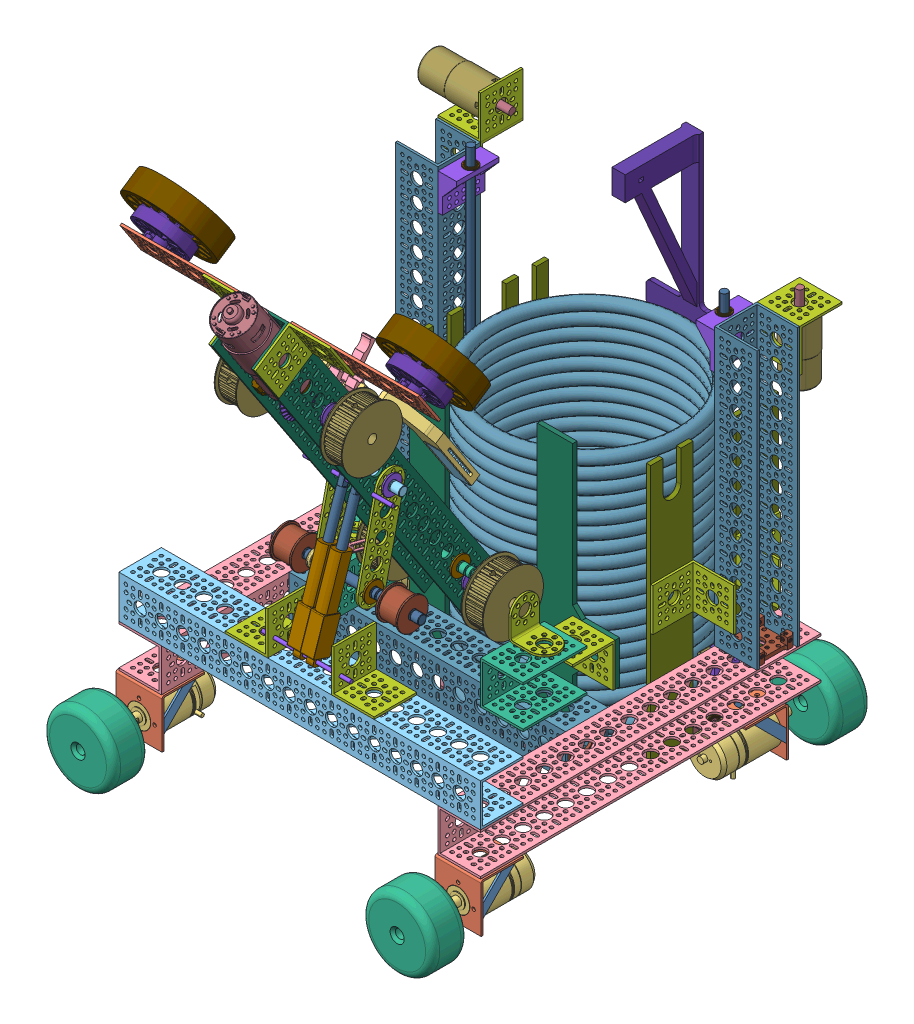
SolidWorks assembly 底座3.5, configuration 默认. Lengths in mm. (continued)
Mates (geometry in assembly coordinates): (continued)
- Concentric323: concentric aligned: cylinder of 升降轴-1 through (7.3414 252.9349 701.0171) axis (-1 0 0) radius 2; cylinder of 电动推杆01-1 through (-46.1586 252.9349 701.0171) axis (-1 0 0) radius 2
- Concentric324: concentric aligned: cylinder of 升降轴-1 through (7.3414 252.9349 701.0171) axis (-1 0 0) radius 2; cylinder of 电动推杆01-2 through (-31.1586 252.9349 701.0171) axis (-1 0 0) radius 2
- Concentric325: concentric anti-aligned: cylinder of 电动推杆01-2 through (-35.1586 294.1889 687.2204) axis (0 0.94837 -0.317167) radius 4.5; cylinder of 电动推杆2-1 through (-35.1586 393.1181 654.1351) axis (0 -0.94837 0.317167) radius 4.5
- LimitDistance1: limit distance = 5.6851 mm anti-aligned: plane of 电动推杆2-1 through (-35.1586 340.9577 671.5793) normal (0 -0.94837 0.317167); plane of 电动推杆01-2 through (-35.1586 346.3493 669.7762) normal (0 0.94837 -0.317167)
- LimitDistance2: limit distance = 49.3149 mm aligned: plane of 电动推杆2-1 through (-35.1586 393.1181 654.1351) normal (0 0.94837 -0.317167); plane of 电动推杆01-2 through (-35.1586 346.3493 669.7762) normal (0 0.94837 -0.317167)
- Concentric328: concentric anti-aligned: cylinder of 电动推杆01-1 through (-50.1586 294.1889 687.2204) axis (0 0.94837 -0.317167) radius 4.5; cylinder of 电动推杆2-2 through (-50.1586 393.1181 654.1351) axis (0 -0.94837 0.317167) radius 4.5
- LimitDistance6: limit distance = 5.6851 mm anti-aligned: plane of 电动推杆01-1 through (-50.1586 346.3493 669.7762) normal (0 0.94837 -0.317167); plane of 电动推杆2-2 through (-50.1586 340.9577 671.5793) normal (0 -0.94837 0.317167)
- LimitDistance7: limit distance = 49.3149 mm aligned: plane of 电动推杆2-2 through (-50.1586 393.1181 654.1351) normal (0 0.94837 -0.317167); plane of 电动推杆01-1 through (-50.1586 346.3493 669.7762) normal (0 0.94837 -0.317167)
- Coincident131: coincident anti-aligned: plane of 电动推杆01-1 through (-42.6586 291.0173 677.7367) normal (1 0 0); plane of 电动推杆01-2 through (-42.6586 297.3606 696.7041) normal (-1 0 0)
- Distance12: distance = 21 mm anti-aligned: plane of 电动推杆01-1 through (-57.6586 297.3606 696.7041) normal (-1 0 0); plane of 48x48-L形支架-3 through (-78.6586 237.4201 661.5024) normal (1 0 0)
- Coincident286: coincident anti-aligned: plane of 384mm-U型梁-2 through (161.3414 189.4201 325.5024) normal (0 1 0); plane of 电机转向座-9 through (137.3414 189.4201 373.5024) normal (0 -1 0)
- Concentric623: concentric anti-aligned: cylinder of 48x48-L形支架-17 through (137.3414 491.4201 325.5024) axis (0 1 0) radius 7; cylinder of 一级摩擦轮电机01-2 through (137.3414 498.9201 325.5024) axis (0 -1 0) radius 11
- Coincident301: coincident anti-aligned: plane of 48x48-L形支架-17 through (113.3414 498.9201 347.0024) normal (0 -1 0); plane of 一级摩擦轮电机01-2 through (137.3414 498.9201 325.5024) normal (0 1 0)
- Tangent10: tangent anti-aligned: plane of 48x48-L形支架-17 through (135.3414 491.4201 347.0024) normal (1 0 0); cylinder of 一级摩擦轮电机01-2 through (136.8414 491.6201 311.5113) axis (0 1 0) radius 1.5
- Concentric624: concentric anti-aligned: cylinder of 一级摩擦轮电机01-2 through (137.3414 495.9201 325.5024) axis (0 1 0) radius 4; cylinder of 一级摩擦轮电机02-2 through (137.3414 515.9201 325.5024) axis (0 -1 0) radius 4
- Coincident302: coincident anti-aligned: plane of 一级摩擦轮电机01-2 through (137.3414 495.9201 325.5024) normal (0 1 0); plane of 一级摩擦轮电机02-2 through (137.3414 495.9201 325.5024) normal (0 -1 0)
- Concentric637: concentric aligned: cylinder of 384mm-U型梁-1 through (-222.6586 179.4201 373.5024) axis (0 1 0) radius 7; cylinder of 电机转向座-12 through (-222.6586 189.4201 373.5024) axis (0 1 0) radius 7
- Concentric638: concentric aligned: cylinder of 384mm-U型梁-2 through (137.3414 179.4201 373.5024) axis (0 1 0) radius 7; cylinder of 电机转向座-9 through (137.3414 189.4201 373.5024) axis (0 1 0) radius 7
- Coincident316: coincident aligned: plane of 384mm-U型梁-2 through (161.3414 189.4201 325.5024) normal (0 1 0); plane of 312mm-U型梁-7 through (113.3414 189.4201 565.5024) normal (0 1 0)
- Coincident317: coincident anti-aligned: plane of 384mm-U型梁-2 through (113.3414 189.4201 325.5024) normal (-1 0 0); plane of 312mm-U型梁-7 through (113.3414 186.9201 541.5024) normal (1 0 0)
- Concentric650: concentric anti-aligned: cylinder of 312mm-U型梁-7 through (105.3414 179.4201 557.5024) axis (0 1 0) radius 2; cone of 电机转向座-13 through (105.3414 186.9201 557.5024) axis (0 -1 0)
- Concentric651: concentric anti-aligned: cylinder of 312mm-U型梁-7 through (105.3414 179.4201 525.5024) axis (0 1 0) radius 2; cone of 电机转向座-13 through (105.3414 186.9201 525.5024) axis (0 -1 0)
- Concentric652: concentric anti-aligned: cylinder of 312mm-U型梁-7 through (105.3414 181.4201 527.5024) axis (0 0 -1) radius 2; cone of 电机转向座-13 through (105.3414 181.4201 520.0024) axis (0 0 1)
- Concentric653: concentric anti-aligned: cylinder of 312mm-U型梁-7 through (105.3414 149.4201 527.5024) axis (0 0 -1) radius 2; cone of 电机转向座-13 through (105.3414 149.4201 520.0024) axis (0 0 1)
- Coincident318: coincident anti-aligned: plane of 384mm-U型梁-2 through (113.3414 189.4201 325.5024) normal (-1 0 0); plane of 电机转向座-13 through (113.3414 165.4201 541.5024) normal (1 0 0)
- Concentric654: concentric aligned: cylinder of 384mm-U型梁-2 through (123.3414 165.4201 541.5024) axis (-1 0 0) radius 7; cylinder of 电机转向座-13 through (113.3414 165.4201 541.5024) axis (-1 0 0) radius 7
- Concentric655: concentric aligned: cylinder of 384mm-U型梁-2 through (123.3414 156.9349 533.0171) axis (-1 0 0) radius 2; cylinder of 电机转向座-13 through (109.3414 156.9349 533.0171) axis (-1 0 0) radius 2
- Concentric661: concentric anti-aligned: cylinder of 312mm-U型梁-7 through (65.3414 179.4201 541.5024) axis (0 1 0) radius 7; cylinder of 72mm-U型梁-5 through (65.3414 199.4201 541.5024) axis (0 -1 0) radius 7
- Coincident323: coincident anti-aligned: plane of 312mm-U型梁-7 through (113.3414 189.4201 565.5024) normal (0 1 0); plane of 72mm-U型梁-5 through (89.3414 189.4201 589.5024) normal (0 -1 0)
- Concentric662: concentric anti-aligned: cylinder of 312mm-U型梁-7 through (81.3414 179.4201 557.5024) axis (0 1 0) radius 2; cylinder of 72mm-U型梁-5 through (81.3414 199.4201 557.5024) axis (0 -1 0) radius 2
- Coincident324: coincident anti-aligned: plane of 312mm-U型梁-7 through (113.3414 189.4201 565.5024) normal (0 1 0); plane of 72mm-U型梁-6 through (-174.6586 189.4201 589.5024) normal (0 -1 0)
- Concentric666: concentric aligned: cylinder of 72mm-U型梁-5 through (65.3414 227.4201 541.5024) axis (0 1 0) radius 7; cylinder of 圆角90°法兰-7 through (65.3414 237.4201 541.5024) axis (0 1 0) radius 7
- Coincident325: coincident anti-aligned: plane of 72mm-U型梁-5 through (89.3414 237.4201 589.5024) normal (0 1 0); plane of 圆角90°法兰-7 through (41.3414 237.4201 557.5024) normal (0 -1 0)
- Concentric667: concentric aligned: cylinder of 72mm-U型梁-5 through (54.0277 234.4201 541.5024) axis (0 1 0) radius 2; cylinder of 圆角90°法兰-7 through (54.0277 237.4201 541.5024) axis (0 1 0) radius 2.025
- Coincident326: coincident anti-aligned: plane of 72mm-U型梁-6 through (-174.6586 237.4201 589.5024) normal (0 1 0); plane of 圆角90°法兰-8 through (-126.6586 237.4201 525.5024) normal (0 -1 0)
- Concentric670: concentric anti-aligned: cylinder of 总装-2/同步轮四十齿(1)-3 through (30.3158 261.4201 541.5024) axis (-1 0 0) radius 5; cylinder of 圆角90°法兰-7 through (41.3414 261.4201 541.5024) axis (1 0 0) radius 7
- Distance14: distance = 12.71 mm anti-aligned: plane of 总装-2/同步轮四十齿(1)-1 through (-113.9486 261.4201 541.5024) normal (-1 0 0); plane of 圆角90°法兰-8 through (-126.6586 237.4201 525.5024) normal (1 0 0)
- Concentric673: concentric anti-aligned: circle of 电动推杆2-1; cylinder of 升降轴-2 through (5.3414 399.2825 652.0735) axis (-1 0 0) radius 2
- Concentric674: concentric anti-aligned: circle of 电动推杆2-2; cylinder of 升降轴-2 through (5.3414 399.2825 652.0735) axis (-1 0 0) radius 2
- Concentric675: concentric aligned: cylinder of 升降轴-2 through (5.3414 399.2825 652.0735) axis (-1 0 0) radius 2; cylinder of 总装-2/432mm-U型梁-1 through (-55.4486 399.2825 652.0735) axis (-1 0 0) radius 2
- Coincident329: coincident anti-aligned: plane of 384mm-U型梁-1 through (-246.6586 189.4201 325.5024) normal (0 1 0); plane of 电机转向座-12 through (-222.6586 189.4201 373.5024) normal (0 -1 0)
- Concentric678: concentric aligned: cylinder of 轴承座-1 through (100.3414 497.4201 373.5024) axis (0 -1 0) radius 7; cylinder of 8-14轴承-7 through (100.3414 497.4201 373.5024) axis (0 -1 0) radius 7
- Coincident330: coincident anti-aligned: plane of 轴承座-1 through (113.3414 497.4201 397.5024) normal (0 1 0); plane of 8-14轴承-7 through (100.3414 497.4201 373.5024) normal (0 -1 0)
- Coincident331: coincident anti-aligned: plane of 384mm-U型梁-2 through (113.3414 189.4201 325.5024) normal (-1 0 0); plane of 轴承座-2 through (113.3414 145.4201 397.5024) normal (1 0 0)
- Concentric679: concentric anti-aligned: cylinder of 384mm-U型梁-2 through (123.3414 181.4201 389.5024) axis (-1 0 0) radius 2; cylinder of 轴承座-2 through (95.3414 181.4201 389.5024) axis (1 0 0) radius 2.05
- Concentric680: concentric anti-aligned: cylinder of 384mm-U型梁-2 through (123.3414 181.4201 357.5024) axis (-1 0 0) radius 2; cylinder of 轴承座-2 through (95.3414 181.4201 357.5024) axis (1 0 0) radius 2.05
- Concentric681: concentric anti-aligned: cylinder of 轴承座-2 through (100.3414 145.4201 373.5024) axis (0 1 0) radius 7; cylinder of 8-14轴承-8 through (100.3414 150.4201 373.5024) axis (0 -1 0) radius 7
- Coincident332: coincident anti-aligned: plane of 轴承座-2 through (113.3414 150.4201 349.5024) normal (0 1 0); plane of 8-14轴承-8 through (100.3414 150.4201 373.5024) normal (0 -1 0)
- Concentric682: concentric anti-aligned: cylinder of 8-14轴承-8 through (100.3414 146.4201 373.5024) axis (0 1 0) radius 4; cylinder of 螺纹杆-3 through (100.3414 517.4201 373.5024) axis (0 -1 0) radius 4
- Distance15: distance = 20 mm aligned: plane of 螺纹杆-3 through (100.3414 517.4201 373.5024) normal (0 1 0); plane of 轴承座-1 through (113.3414 497.4201 397.5024) normal (0 1 0)
- Concentric684: concentric aligned: cylinder of 螺纹杆-3 through (100.3414 517.4201 373.5024) axis (0 -1 0) radius 4; cylinder of 切边螺纹滑块-1 through (100.3414 168.0411 373.5024) axis (0 -1 0) radius 3.35
- Concentric687: concentric anti-aligned: cylinder of 384mm-U型梁-1 through (-208.6586 181.4201 389.5024) axis (1 0 0) radius 2; cylinder of 轴承座-4 through (-180.6586 181.4201 389.5024) axis (-1 0 0) radius 2.05
- Concentric688: concentric anti-aligned: cylinder of 384mm-U型梁-1 through (-208.6586 181.4201 357.5024) axis (1 0 0) radius 2; cylinder of 轴承座-4 through (-180.6586 181.4201 357.5024) axis (-1 0 0) radius 2.05
- Coincident334: coincident anti-aligned: plane of 384mm-U型梁-1 through (-198.6586 141.4201 325.5024) normal (1 0 0); plane of 轴承座-4 through (-198.6586 145.4201 349.5024) normal (-1 0 0)
- Concentric689: concentric aligned: cylinder of 轴承座-3 through (-185.6586 497.4201 373.5024) axis (0 -1 0) radius 7; cylinder of 8-14轴承-9 through (-185.6586 497.4201 373.5024) axis (0 -1 0) radius 7
- Coincident335: coincident anti-aligned: plane of 轴承座-3 through (-198.6586 497.4201 349.5024) normal (0 1 0); plane of 8-14轴承-9 through (-185.6586 497.4201 373.5024) normal (0 -1 0)
- Concentric690: concentric anti-aligned: cylinder of 轴承座-4 through (-185.6586 145.4201 373.5024) axis (0 1 0) radius 7; cylinder of 8-14轴承-10 through (-185.6586 150.4201 373.5024) axis (0 -1 0) radius 7
- Coincident336: coincident anti-aligned: plane of 轴承座-4 through (-198.6586 150.4201 397.5024) normal (0 1 0); plane of 8-14轴承-10 through (-185.6586 150.4201 373.5024) normal (0 -1 0)
- Concentric691: concentric anti-aligned: cylinder of 8-14轴承-9 through (-185.6586 493.4201 373.5024) axis (0 1 0) radius 4; cylinder of 螺纹杆-4 through (-185.6586 517.4201 373.5024) axis (0 -1 0) radius 4
- Coincident337: coincident aligned: plane of 螺纹杆-3 through (100.3414 517.4201 373.5024) normal (0 1 0); plane of 螺纹杆-4 through (-185.6586 517.4201 373.5024) normal (0 1 0)
- Concentric692: concentric aligned: cylinder of 螺纹杆-4 through (-185.6586 517.4201 373.5024) axis (0 -1 0) radius 4; cylinder of 切边螺纹滑块-2 through (-185.6586 168.0411 373.5024) axis (0 -1 0) radius 3.35
- Coincident338: coincident aligned: plane of 切边螺纹滑块-1 through (100.3414 158.0411 373.5024) normal (0 1 0); plane of 切边螺纹滑块-2 through (-185.6586 158.0411 373.5024) normal (0 1 0)
- Concentric693: concentric anti-aligned: cylinder of 切边螺纹滑块-1 through (100.3414 153.0411 373.5024) axis (0 1 0) radius 5.1; cylinder of 转换块-1 through (100.3414 163.0411 373.5024) axis (0 -1 0) radius 5.5
- Concentric694: concentric aligned: cylinder of 切边螺纹滑块-1 through (100.3414 158.0411 365.5024) axis (0 -1 0) radius 1.75; cylinder of 转换块-1 through (100.3414 163.0411 365.5024) axis (0 -1 0) radius 1.75
- Coincident339: coincident anti-aligned: plane of 切边螺纹滑块-1 through (100.3414 158.0411 373.5024) normal (0 1 0); plane of 转换块-1 through (100.3414 158.0411 373.5024) normal (0 -1 0)
- Concentric695: concentric anti-aligned: cylinder of 切边螺纹滑块-2 through (-185.6586 153.0411 373.5024) axis (0 1 0) radius 5.1; cylinder of 转换块-2 through (-185.6586 163.0411 373.5024) axis (0 -1 0) radius 5.5
- Concentric696: concentric aligned: cylinder of 切边螺纹滑块-2 through (-185.6586 158.0411 365.5024) axis (0 -1 0) radius 1.75; cylinder of 转换块-2 through (-185.6586 163.0411 365.5024) axis (0 -1 0) radius 1.75
- Coincident340: coincident anti-aligned: plane of 切边螺纹滑块-2 through (-185.6586 158.0411 373.5024) normal (0 1 0); plane of 转换块-2 through (-185.6586 158.0411 373.5024) normal (0 -1 0)
- Concentric697: concentric aligned: cylinder of 384mm-U型梁-2 through (121.3414 179.4201 365.5024) axis (0 1 0) radius 2; cylinder of 电机转向座-9 through (121.3414 193.4201 365.5024) axis (0 1 0) radius 2
- Concentric698: concentric anti-aligned: cone of 电机转向座-9 through (121.3414 197.4201 352.0024) axis (0 0 1); cylinder of 312mm-U型梁-8 through (121.3414 197.4201 359.5024) axis (0 0 -1) radius 2
- Concentric699: concentric anti-aligned: cone of 电机转向座-9 through (153.3414 197.4201 352.0024) axis (0 0 1); cylinder of 312mm-U型梁-8 through (153.3414 197.4201 359.5024) axis (0 0 -1) radius 2
- Concentric700: concentric anti-aligned: cone of 电机转向座-9 through (116.1914 197.4201 357.5024) axis (1 0 0); cylinder of 312mm-U型梁-8 through (123.3414 197.4201 357.5024) axis (-1 0 0) radius 2
- Concentric701: concentric anti-aligned: cone of 电机转向座-9 through (116.1914 197.4201 389.5024) axis (1 0 0); cylinder of 312mm-U型梁-8 through (123.3414 197.4201 389.5024) axis (-1 0 0) radius 2
- Coincident341: coincident anti-aligned: plane of 轴承座-1 through (113.3414 497.4201 349.5024) normal (1 0 0); plane of 312mm-U型梁-8 through (113.3414 189.4201 349.5024) normal (-1 0 0)
- Concentric704: concentric anti-aligned: cylinder of 48x48-L形支架-17 through (153.3414 493.4201 339.5024) axis (0 0 1) radius 2; cylinder of 312mm-U型梁-8 through (153.3414 493.4201 359.5024) axis (0 0 -1) radius 2
- Concentric705: concentric anti-aligned: cylinder of 48x48-L形支架-17 through (121.3414 493.4201 339.5024) axis (0 0 1) radius 2; cylinder of 312mm-U型梁-8 through (121.3414 493.4201 359.5024) axis (0 0 -1) radius 2
- Coincident342: coincident anti-aligned: plane of 48x48-L形支架-17 through (113.3414 501.4201 349.5024) normal (0 0 1); plane of 312mm-U型梁-8 through (161.3414 189.4201 349.5024) normal (0 0 -1)
- Concentric706: concentric anti-aligned: cylinder of 轴承座-1 through (95.3414 477.4201 357.5024) axis (1 0 0) radius 2.05; cylinder of 312mm-U型梁-8 through (123.3414 477.4201 357.5024) axis (-1 0 0) radius 2
- Concentric707: concentric anti-aligned: cylinder of 轴承座-1 through (95.3414 477.4201 389.5024) axis (1 0 0) radius 2.05; cylinder of 312mm-U型梁-8 through (123.3414 477.4201 389.5024) axis (-1 0 0) radius 2
- Concentric708: concentric aligned: cylinder of 384mm-U型梁-1 through (-206.6586 179.4201 365.5024) axis (0 1 0) radius 2; cylinder of 电机转向座-12 through (-206.6586 193.4201 365.5024) axis (0 1 0) radius 2
- Concentric709: concentric anti-aligned: cone of 电机转向座-12 through (-238.6586 197.4201 352.0024) axis (0 0 1); cylinder of 312mm-U型梁-9 through (-238.6586 197.4201 359.5024) axis (0 0 -1) radius 2
- Concentric710: concentric anti-aligned: cone of 电机转向座-12 through (-206.6586 197.4201 352.0024) axis (0 0 1); cylinder of 312mm-U型梁-9 through (-206.6586 197.4201 359.5024) axis (0 0 -1) radius 2
- Concentric711: concentric anti-aligned: cone of 电机转向座-12 through (-201.1586 197.4201 357.5024) axis (-1 0 0); cylinder of 312mm-U型梁-9 through (-208.6586 197.4201 357.5024) axis (1 0 0) radius 2
- Concentric712: concentric anti-aligned: cone of 电机转向座-12 through (-201.1586 197.4201 389.5024) axis (-1 0 0); cylinder of 312mm-U型梁-9 through (-208.6586 197.4201 389.5024) axis (1 0 0) radius 2
- Concentric713: concentric anti-aligned: cylinder of 48x48-L形支架-18 through (-206.6586 493.4201 339.5024) axis (0 0 1) radius 2; cylinder of 312mm-U型梁-9 through (-206.6586 493.4201 359.5024) axis (0 0 -1) radius 2
- Concentric714: concentric anti-aligned: cylinder of 48x48-L形支架-18 through (-238.6586 493.4201 339.5024) axis (0 0 1) radius 2; cylinder of 312mm-U型梁-9 through (-238.6586 493.4201 359.5024) axis (0 0 -1) radius 2
- Coincident343: coincident anti-aligned: plane of 48x48-L形支架-18 through (-246.6586 501.4201 349.5024) normal (0 0 1); plane of 312mm-U型梁-9 through (-246.6586 189.4201 349.5024) normal (0 0 -1)
- Concentric715: concentric anti-aligned: cylinder of 轴承座-3 through (-180.6586 477.4201 357.5024) axis (-1 0 0) radius 2.05; cylinder of 312mm-U型梁-9 through (-208.6586 477.4201 357.5024) axis (1 0 0) radius 2
- Concentric716: concentric anti-aligned: cylinder of 轴承座-3 through (-180.6586 477.4201 389.5024) axis (-1 0 0) radius 2.05; cylinder of 312mm-U型梁-9 through (-208.6586 477.4201 389.5024) axis (1 0 0) radius 2
- Coincident344: coincident anti-aligned: plane of 轴承座-3 through (-198.6586 497.4201 397.5024) normal (-1 0 0); plane of 312mm-U型梁-9 through (-198.6586 189.4201 397.5024) normal (1 0 0)
- Parallel5: parallel aligned: plane of 转换块-1 through (82.3414 163.0411 361.5024) normal (-1 0 0); plane of 312mm-U型梁-8 through (113.3414 189.4201 349.5024) normal (-1 0 0)
- Parallel6: parallel aligned: plane of 转换块-2 through (-167.6586 163.0411 385.5024) normal (1 0 0); plane of 312mm-U型梁-9 through (-198.6586 189.4201 397.5024) normal (1 0 0)
- Concentric717: concentric aligned: cylinder of 转换块-1 through (142.3414 90.0411 373.5024) axis (-1 0 0) radius 7; cylinder of 8-14轴承-11 through (87.3414 90.0411 373.5024) axis (-1 0 0) radius 7
- Coincident345: coincident anti-aligned: plane of 转换块-1 through (87.3414 78.0411 361.5024) normal (1 0 0); plane of 8-14轴承-11 through (87.3414 90.0411 373.5024) normal (-1 0 0)
- Concentric718: concentric aligned: cylinder of 转换块-2 through (-227.6586 90.0411 373.5024) axis (1 0 0) radius 7; cylinder of 8-14轴承-12 through (-172.6586 90.0411 373.5024) axis (1 0 0) radius 7
- Coincident346: coincident anti-aligned: plane of 转换块-2 through (-172.6586 78.0411 385.5024) normal (-1 0 0); plane of 8-14轴承-12 through (-172.6586 90.0411 373.5024) normal (1 0 0)
- Concentric719: concentric aligned: cylinder of 8-14轴承-11 through (83.3414 90.0411 373.5024) axis (1 0 0) radius 4; cylinder of 铲板-1 through (-164.6586 90.0411 373.5024) axis (1 0 0) radius 6
- Coincident347: coincident anti-aligned: plane of 8-14轴承-11 through (83.3414 90.0411 373.5024) normal (-1 0 0); plane of 铲板-1 through (83.3414 90.0411 373.5024) normal (1 0 0)
- Concentric720: concentric aligned: cylinder of 72mm-U型梁-6 through (-150.6586 227.4201 541.5024) axis (0 1 0) radius 7; cylinder of 圆角90°法兰-8 through (-150.6586 237.4201 541.5024) axis (0 1 0) radius 7
- Concentric721: concentric anti-aligned: cylinder of 312mm-U型梁-7 through (-150.6586 179.4201 541.5024) axis (0 1 0) radius 7; cylinder of 72mm-U型梁-6 through (-150.6586 199.4201 541.5024) axis (0 -1 0) radius 7
- Concentric727: concentric anti-aligned: cylinder of 312mm-U型梁-7 through (-166.6586 179.4201 525.5024) axis (0 1 0) radius 2; cylinder of 72mm-U型梁-6 through (-166.6586 199.4201 525.5024) axis (0 -1 0) radius 2
- Concentric728: concentric aligned: cylinder of 72mm-U型梁-6 through (-150.6586 234.4201 530.1887) axis (0 1 0) radius 2; cylinder of 圆角90°法兰-8 through (-150.6586 237.4201 530.1887) axis (0 1 0) radius 2.025
- Coincident353: coincident anti-aligned: plane of 72mm-U型梁-6 through (-129.1586 234.9201 589.5024) normal (0 -1 0); plane of 48x48-L形支架-20 through (-182.6586 234.9201 493.5024) normal (0 1 0)
- Concentric736: concentric aligned: cylinder of 72mm-U型梁-6 through (-166.6586 227.4201 533.5024) axis (0 1 0) radius 2; cylinder of 48x48-L形支架-20 through (-166.6586 224.9201 533.5024) axis (0 1 0) radius 2
- Concentric737: concentric aligned: cylinder of 72mm-U型梁-6 through (-166.6586 227.4201 525.5024) axis (0 1 0) radius 2; cylinder of 48x48-L形支架-20 through (-166.6586 224.9201 525.5024) axis (0 1 0) radius 2
- Concentric738: concentric anti-aligned: cylinder of 48x48-L形支架-20 through (-158.6586 210.9201 503.5024) axis (0 0 -1) radius 7; cylinder of 前挡板-1 through (-158.6586 210.9201 488.5024) axis (0 0 1) radius 7
- Coincident354: coincident anti-aligned: plane of 48x48-L形支架-20 through (-182.6586 186.9201 493.5024) normal (0 0 -1); plane of 前挡板-1 through (-94.6586 402.9201 493.5024) normal (0 0 1)
- Concentric739: concentric anti-aligned: cylinder of 48x48-L形支架-20 through (-174.6586 226.9201 503.5024) axis (0 0 -1) radius 2; cylinder of 前挡板-1 through (-174.6586 226.9201 488.5024) axis (0 0 1) radius 2
- Coincident356: coincident anti-aligned: plane of 312mm-U型梁-9 through (-246.6586 189.4201 397.5024) normal (0 0 1); plane of 48x48-L形支架-22 through (-174.6586 213.4201 397.5024) normal (0 0 -1)
- Concentric742: concentric anti-aligned: cylinder of 312mm-U型梁-9 through (-206.6586 253.4201 387.5024) axis (0 0 1) radius 2; cylinder of 48x48-L形支架-22 through (-206.6586 253.4201 407.5024) axis (0 0 -1) radius 2
- Concentric743: concentric anti-aligned: cylinder of 312mm-U型梁-9 through (-214.6586 253.4201 387.5024) axis (0 0 1) radius 2; cylinder of 48x48-L形支架-22 through (-214.6586 253.4201 407.5024) axis (0 0 -1) radius 2
- Coincident357: coincident anti-aligned: plane of 312mm-U型梁-9 through (-246.6586 189.4201 349.5024) normal (0 0 -1); plane of 48x48-L形支架-23 through (-174.6586 261.4201 349.5024) normal (0 0 1)
- Concentric744: concentric anti-aligned: cylinder of 312mm-U型梁-9 through (-206.6586 253.4201 359.5024) axis (0 0 -1) radius 2; cylinder of 48x48-L形支架-23 through (-206.6586 253.4201 339.5024) axis (0 0 1) radius 2
- Concentric745: concentric anti-aligned: cylinder of 312mm-U型梁-9 through (-214.6586 253.4201 359.5024) axis (0 0 -1) radius 2; cylinder of 48x48-L形支架-23 through (-214.6586 253.4201 339.5024) axis (0 0 1) radius 2
- Concentric746: concentric anti-aligned: cylinder of 48x48-L形支架-23 through (-184.6586 237.4201 325.5024) axis (1 0 0) radius 7; cylinder of 侧挡板-1 through (-169.6586 237.4201 325.5024) axis (-1 0 0) radius 7
- Coincident358: coincident anti-aligned: plane of 48x48-L形支架-23 through (-174.6586 261.4201 301.5024) normal (1 0 0); plane of 侧挡板-1 through (-174.6586 77.4201 301.5024) normal (-1 0 0)
- Concentric747: concentric anti-aligned: cylinder of 48x48-L形支架-23 through (-184.6586 253.4201 341.5024) axis (1 0 0) radius 2; cylinder of 侧挡板-1 through (-169.6586 253.4201 341.5024) axis (-1 0 0) radius 2
- Concentric748: concentric anti-aligned: cylinder of 48x48-L形支架-22 through (-184.6586 237.4201 421.5024) axis (1 0 0) radius 7; cylinder of 侧挡板-2 through (-169.6586 237.4201 421.5024) axis (-1 0 0) radius 7
- Concentric749: concentric anti-aligned: cylinder of 48x48-L形支架-22 through (-184.6586 253.4201 437.5024) axis (1 0 0) radius 2; cylinder of 侧挡板-2 through (-169.6586 253.4201 437.5024) axis (-1 0 0) radius 2
- Coincident359: coincident anti-aligned: plane of 48x48-L形支架-22 through (-174.6586 213.4201 445.5024) normal (1 0 0); plane of 侧挡板-2 through (-174.6586 77.4201 397.5024) normal (-1 0 0)
- Coincident360: coincident anti-aligned: plane of 312mm-U型梁-8 through (161.3414 189.4201 349.5024) normal (0 0 -1); plane of 48x48-L形支架-24 through (137.3414 261.4201 349.5024) normal (0 0 1)
- Concentric750: concentric anti-aligned: cylinder of 312mm-U型梁-8 through (121.3414 253.4201 359.5024) axis (0 0 -1) radius 2; cylinder of 48x48-L形支架-24 through (121.3414 253.4201 339.5024) axis (0 0 1) radius 2
- Concentric751: concentric anti-aligned: cylinder of 312mm-U型梁-8 through (129.3414 253.4201 359.5024) axis (0 0 -1) radius 2; cylinder of 48x48-L形支架-24 through (129.3414 253.4201 339.5024) axis (0 0 1) radius 2
- Concentric752: concentric aligned: cylinder of 侧挡板-3 through (89.3414 237.4201 325.5024) axis (-1 0 0) radius 7; cylinder of 48x48-L形支架-24 through (99.3414 237.4201 325.5024) axis (-1 0 0) radius 7
- Coincident361: coincident anti-aligned: plane of 侧挡板-3 through (89.3414 77.4201 301.5024) normal (1 0 0); plane of 48x48-L形支架-24 through (89.3414 261.4201 349.5024) normal (-1 0 0)
- Concentric753: concentric aligned: cylinder of 侧挡板-3 through (89.3414 253.4201 309.5024) axis (-1 0 0) radius 2; cylinder of 48x48-L形支架-24 through (99.3414 253.4201 309.5024) axis (-1 0 0) radius 2
- Coincident362: coincident anti-aligned: plane of 312mm-U型梁-8 through (161.3414 189.4201 397.5024) normal (0 0 1); plane of 48x48-L形支架-25 through (89.3414 261.4201 397.5024) normal (0 0 -1)
- Concentric754: concentric anti-aligned: cylinder of 312mm-U型梁-8 through (121.3414 253.4201 387.5024) axis (0 0 1) radius 2; cylinder of 48x48-L形支架-25 through (121.3414 253.4201 407.5024) axis (0 0 -1) radius 2
- Concentric755: concentric anti-aligned: cylinder of 312mm-U型梁-8 through (129.3414 253.4201 387.5024) axis (0 0 1) radius 2; cylinder of 48x48-L形支架-25 through (129.3414 253.4201 407.5024) axis (0 0 -1) radius 2
- Concentric756: concentric aligned: cylinder of 侧挡板-4 through (89.3414 237.4201 421.5024) axis (-1 0 0) radius 7; cylinder of 48x48-L形支架-25 through (99.3414 237.4201 421.5024) axis (-1 0 0) radius 7
- Coincident363: coincident anti-aligned: plane of 侧挡板-4 through (89.3414 77.4201 397.5024) normal (1 0 0); plane of 48x48-L形支架-25 through (89.3414 261.4201 445.5024) normal (-1 0 0)
- Concentric757: concentric aligned: cylinder of 侧挡板-4 through (89.3414 253.4201 437.5024) axis (-1 0 0) radius 2; cylinder of 48x48-L形支架-25 through (99.3414 253.4201 437.5024) axis (-1 0 0) radius 2
- Coincident364: coincident anti-aligned: plane of 72mm-U型梁-5 through (43.8414 234.9201 589.5024) normal (0 -1 0); plane of 48x48-L形支架-26 through (49.3414 234.9201 493.5024) normal (0 1 0)
- Concentric758: concentric aligned: cylinder of 72mm-U型梁-5 through (81.3414 227.4201 533.5024) axis (0 1 0) radius 2; cylinder of 48x48-L形支架-26 through (81.3414 224.9201 533.5024) axis (0 1 0) radius 2
- Concentric759: concentric aligned: cylinder of 72mm-U型梁-5 through (81.3414 227.4201 525.5024) axis (0 1 0) radius 2; cylinder of 48x48-L形支架-26 through (81.3414 224.9201 525.5024) axis (0 1 0) radius 2
- Coincident365: coincident anti-aligned: plane of 48x48-L形支架-26 through (49.3414 186.9201 493.5024) normal (0 0 -1); plane of 前挡板-2 through (9.3414 402.9201 493.5024) normal (0 0 1)
- Concentric760: concentric aligned: cylinder of 48x48-L形支架-26 through (73.3414 210.9201 503.5024) axis (0 0 -1) radius 7; cylinder of 前挡板-2 through (73.3414 210.9201 493.5024) axis (0 0 -1) radius 7
- Concentric761: concentric aligned: cylinder of 48x48-L形支架-26 through (89.3414 194.9201 503.5024) axis (0 0 -1) radius 2; cylinder of 前挡板-2 through (89.3414 194.9201 493.5024) axis (0 0 -1) radius 2
- 重合1: coincident anti-aligned: plane of 一级摩擦轮电机02-3 through (-206.7756 525.4201 325.5024) normal (-1 0 0); plane of 一级摩擦轮电机01-4 through (-206.7756 525.4201 325.5024) normal (1 0 0)
- 重合2: coincident aligned: circle of 一级摩擦轮电机02-3; circle of 一级摩擦轮电机01-4
- 重合3: coincident anti-aligned: circle of 48x48-L形支架-18; circle of 48x48-L形支架-27
- 重合4: coincident aligned: plane of 48x48-L形支架-18 through (-198.6586 477.4201 347.0024) normal (1 0 0); plane of 48x48-L形支架-27 through (-198.6586 501.4201 301.5024) normal (1 0 0)
- 同心1: concentric anti-aligned: circle of 一级摩擦轮电机02-3; circle of 48x48-L形支架-27
